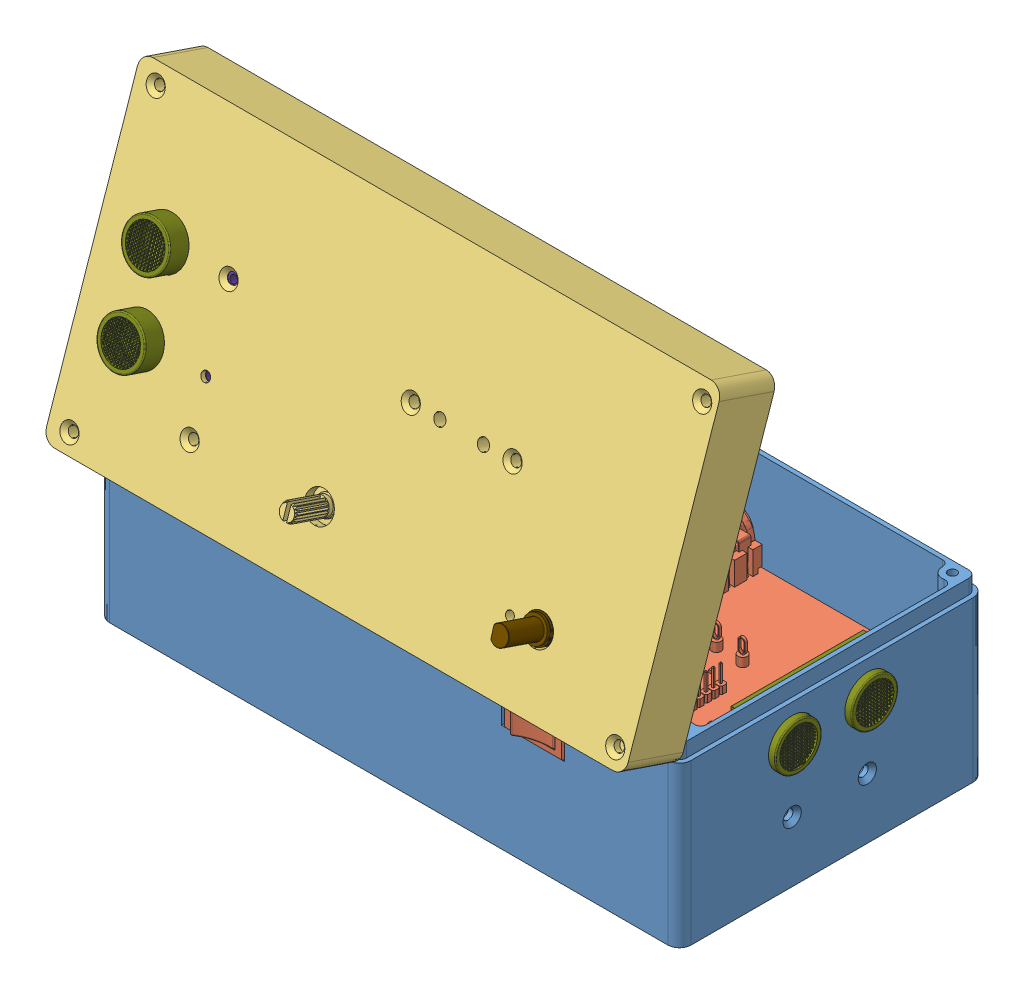
SolidWorks assembly Assemblage_Theremin, configuration Default. Lengths in mm.
Overall size (203.87 162.26 138.46).
66 component instances, 21 part files, 15 mates.
Components (placement in the parent):
- Theremin-Boitier_JonathanCHAFLA-1: Theremin-Boitier_JonathanCHAFLA [Default] at (-1328.4654 62.0969 1104.789) size (203 60 108)
- Theremin_PCB-Chafla.step-2: Theremin_PCB-Chafla.step [Default] at (-1384.7495 88.7032 1147.6303) x (1 0 0) z (0 1 0) size (155 102.12 38.23)
- Theremin-Boitier_JonathanCHAFLA-Couvercle-1: Theremin-Boitier_JonathanCHAFLA-Couvercle [Default] at (-1327.4934 174.761 1150.8521) x (1 0 0) z (0 0.946636 -0.322305) size (203 20 108)
- ThereminPart2_new.step-1: ThereminPart2_new.step [Default] at (-1282.4784 181.7259 1137.917) x (-0.999986 -0.005004 0.001704) z (0 0.322305 0.946636) size (85.91 17.79 19.44)
- PCB_Sensor_V3.step-1: PCB_Sensor_V3.step [Default] at (-1376.0149 146.0045 1153.5546) x (1 0 0) z (0 0.322305 0.946636) size (44.5 45.45 20.31)
  - Board.step-1: Board.step [Default] at origin size (24.5 45 1.61)
    - Open CASCADE STEP translator 6.8 1.1.1.step-1: Open CASCADE STEP translator 6.8 1.1.1.step [Default] at (0 0 -1.6063) size (24.5 45 1.61)
  - X1.step-1: X1.step [Default] at origin size (8.5 10.8 2.5)
    - 6023732704.step-1: 6023732704.step [Default] at (4.275 22.5 1.75) size (8.5 10.8 0.75)
      - Extruded.step-1: Extruded.step [Default] at origin size (8.5 10.8 0.75)
    - 6023732704.step-2: 6023732704.step [Default] at (4.275 22.5 0) size (8.5 10.8 0.75)
      - Extruded.step-1: Extruded.step [Default] at origin size (8.5 10.8 0.75)
    - 6023731264.step-1: 6023731264.step [Default] at (3.925 22.5 0.75) size (7.8 10.8 1)
      - Extruded-1.step-1: Extruded-1.step [Default] at origin size (7.8 10.8 1)
  - X2.step-1: X2.step [Default] at origin size (6.5 8.6 2.25)
    - 686104148922.step-1: 686104148922.step [Default] at (20.5501 22.4999 1.17) x (0 1 0) z (0 0 1) size (8.6 6.5 2.25)
      - 686104148922-0.step-1: 686104148922-0.step [Default] at origin size (8.6 4.5 2.2)
      - 6861xx148922_Patte.step-1: 6861xx148922_Patte.step [Default] at (2.9 0.7 -0.125) x (-1 0 0) z (0 0 1) size (1.4 3.1 1.85)
      - 6861xx148922_Patte2.step-1: 6861xx148922_Patte2.step [Default] at (-3.1 0.7 -0.125) x (-1 0 0) z (0 0 1) size (1.4 3.1 1.85)
      - 6861xx148922_Pin.step-1: 6861xx148922_Pin.step [Default] at (1.6 1.125 0.2986) x (-1 0 0) z (0 0 -1) size (0.2 4.6 2.25)
      - 6861xx148922_Pin.step-2: 6861xx148922_Pin.step [Default] at (0.6 1.125 0.2986) x (-1 0 0) z (0 0 -1) size (0.2 4.6 2.25)
      - 6861xx148922_Pin.step-3: 6861xx148922_Pin.step [Default] at (-0.4 1.125 0.2986) x (-1 0 0) z (0 0 -1) size (0.2 4.6 2.25)
      - 6861xx148922_Pin.step-4: 6861xx148922_Pin.step [Default] at (-1.4 1.125 0.2986) x (-1 0 0) z (0 0 -1) size (0.2 4.6 2.25)
      - 686104148922_Actuator.step-1: 686104148922_Actuator.step [Default] at (0 -2.25 0.4) x (1 0 0) z (0 -1 0) size (8.6 1.4 2.9)
  - C1.step-1: C1.step [Default] at origin size (1.25 2.01 0.94)
    - Cap_AVX_0805YA0R5BAT2A_eec.step-1: Cap_AVX_0805YA0R5BAT2A_eec.step [Default] at (13.5 18 0) x (0 1 0) z (0 0 1) size (2.01 1.25 0.94)
      - Terminals.step-1: Terminals.step [Default] at origin size (2.01 1.25 0.94)
      - Electrode.step-1: Electrode.step [Default] at origin size (1.01 1.25 0.94)
      - AVX.step-1: AVX.step [Default] at origin size (0.37 0.13 0)
  - Free-Models.step-1: Free-Models.step [Default] at origin size (35.25 45.45 20.1)
    - HC-SR04-UltrasonicSensor_v7.step-1: HC-SR04-UltrasonicSensor_v7.step [Default] at (-10 22.5 5.1) x (0 1 0) z (0 0 1) size (45.45 26.2 17.79)
    - 9774100360R_(rev1).step-1: 9774100360R_(rev1).step [Default] at (12.25 9.5 10) x (1 0 0) z (0 1 0) size (6 11.4 6)
    - 9774100360R_(rev1).step-2: 9774100360R_(rev1).step [Default] at (12.25 35.4279 10) x (1 0 0) z (0 1 0) size (6 11.4 6)
- PCB_Sensor_V3 - Copie.step-1: PCB_Sensor_V3 - Copie.step [Default] at (-1223.7904 95.1093 1125.4125) x (0 -1 0.00035) z (1 0 0) size (44.5 45.45 20.31)
  - Board.step-1: Board.step [Default] at origin size (24.5 45 1.61)
    - Open CASCADE STEP translator 6.8 1.1.1.step-1: Open CASCADE STEP translator 6.8 1.1.1.step [Default] at (0 0 -1.6063) size (24.5 45 1.61)
  - X1.step-1: X1.step [Default] at origin size (8.5 10.8 2.5)
    - 6023732704.step-1: 6023732704.step [Default] at (4.275 22.5 1.75) size (8.5 10.8 0.75)
      - Extruded.step-1: Extruded.step [Default] at origin size (8.5 10.8 0.75)
    - 6023732704.step-2: 6023732704.step [Default] at (4.275 22.5 0) size (8.5 10.8 0.75)
      - Extruded.step-1: Extruded.step [Default] at origin size (8.5 10.8 0.75)
    - 6023731264.step-1: 6023731264.step [Default] at (3.925 22.5 0.75) size (7.8 10.8 1)
      - Extruded-1.step-1: Extruded-1.step [Default] at origin size (7.8 10.8 1)
  - X2.step-1: X2.step [Default] at origin size (6.5 8.6 2.25)
    - 686104148922.step-1: 686104148922.step [Default] at (20.5501 22.4999 1.17) x (0 1 0) z (0 0 1) size (8.6 6.5 2.25)
      - 686104148922-0.step-1: 686104148922-0.step [Default] at origin size (8.6 4.5 2.2)
      - 6861xx148922_Patte.step-1: 6861xx148922_Patte.step [Default] at (2.9 0.7 -0.125) x (-1 0 0) z (0 0 1) size (1.4 3.1 1.85)
      - 6861xx148922_Patte2.step-1: 6861xx148922_Patte2.step [Default] at (-3.1 0.7 -0.125) x (-1 0 0) z (0 0 1) size (1.4 3.1 1.85)
      - 6861xx148922_Pin.step-1: 6861xx148922_Pin.step [Default] at (1.6 1.125 0.2986) x (-1 0 0) z (0 0 -1) size (0.2 4.6 2.25)
      - 6861xx148922_Pin.step-2: 6861xx148922_Pin.step [Default] at (0.6 1.125 0.2986) x (-1 0 0) z (0 0 -1) size (0.2 4.6 2.25)
      - 6861xx148922_Pin.step-3: 6861xx148922_Pin.step [Default] at (-0.4 1.125 0.2986) x (-1 0 0) z (0 0 -1) size (0.2 4.6 2.25)
      - 6861xx148922_Pin.step-4: 6861xx148922_Pin.step [Default] at (-1.4 1.125 0.2986) x (-1 0 0) z (0 0 -1) size (0.2 4.6 2.25)
      - 686104148922_Actuator.step-1: 686104148922_Actuator.step [Default] at (0 -2.25 0.4) x (1 0 0) z (0 -1 0) size (8.6 1.4 2.9)
  - C1.step-1: C1.step [Default] at origin size (1.25 2.01 0.94)
    - Cap_AVX_0805YA0R5BAT2A_eec.step-1: Cap_AVX_0805YA0R5BAT2A_eec.step [Default] at (13.5 18 0) x (0 1 0) z (0 0 1) size (2.01 1.25 0.94)
      - Terminals.step-1: Terminals.step [Default] at origin size (2.01 1.25 0.94)
      - Electrode.step-1: Electrode.step [Default] at origin size (1.01 1.25 0.94)
      - AVX.step-1: AVX.step [Default] at origin size (0.37 0.13 0)
  - Free-Models.step-1: Free-Models.step [Default] at origin size (35.25 45.45 20.1)
    - HC-SR04-UltrasonicSensor_v7.step-1: HC-SR04-UltrasonicSensor_v7.step [Default] at (-10 22.5 5.1) x (0 1 0) z (0 0 1) size (45.45 26.2 17.79)
    - 9774100360R_(rev1).step-1: 9774100360R_(rev1).step [Default] at (12.25 9.5 10) x (1 0 0) z (0 1 0) size (6 11.4 6)
    - 9774100360R_(rev1).step-2: 9774100360R_(rev1).step [Default] at (12.25 35.4279 10) x (1 0 0) z (0 1 0) size (6 11.4 6)
- A10405RNZQE_PART1.par-1: A10405RNZQE_PART1.par [Default] at (-1244.4868 141.1795 1153.1092) x (-0.999101 -0.04013 0.013663) z (-0.042392 0.945785 -0.322015) size (26.31 41.71 26.31)
- HP-2: HP [Défaut] at (-1406.4637 94.0969 1104.789) x (0 0 -1) z (1 0 0) size (36 36 16.5)
- jw-s11rww-2: jw-s11rww [Default] at (-1257.7609 105.7894 1152.6396) x (0 -1 0) z (0 0 1) size (15 22 25.64)
- Potentiometer-2: Potentiometer [Default] at (-1319.5713 140.814 1155.6071) x (-1 -0.000493 0.000168) z (-0.000521 0.946636 -0.322305) size (16.35 29.13 24.85)
Mates (geometry in assembly coordinates):
- Coïncidente20: coincident aligned: circle of Theremin-Boitier_JonathanCHAFLA-1; cylinder of PCB_Sensor_V3 - Copie.step-1/Free-Models.step-1/HC-SR04-UltrasonicSensor_v7.step-1 through (-1217.0904 105.0969 1089.789) axis (1 0 0) radius 8
- Coïncidente41: coincident aligned: plane of Theremin-Boitier_JonathanCHAFLA-1 through (-1378.4654 87.0969 1141.789) normal (0 1 0); circle of Theremin_PCB-Chafla.step-2
- Coïncidente76: coincident anti-aligned: line of Theremin-Boitier_JonathanCHAFLA-1 through (-1403.4637 117.0969 1154.6396) axis (1 0 0); line of Theremin-Boitier_JonathanCHAFLA-Couvercle-1 through (-1211.4637 117.0969 1154.6396) axis (-1 0 0)
- Coïncidente77: coincident aligned: plane of Theremin-Boitier_JonathanCHAFLA-1 through (-1207.4637 122.0969 1049.6396) normal (1 0 0); plane of Theremin-Boitier_JonathanCHAFLA-Couvercle-1 through (-1207.4637 123.5429 1173.5723) normal (1 0 0)
- Coïncidente78: coincident aligned: cylinder of Theremin-Boitier_JonathanCHAFLA-Couvercle-1 through (-1386.0149 158.6582 1161.6165) axis (0 -0.322305 -0.946636) radius 8; circle of PCB_Sensor_V3.step-1/Free-Models.step-1/HC-SR04-UltrasonicSensor_v7.step-1
- Coïncidente79: coincident anti-aligned: circle of Theremin-Boitier_JonathanCHAFLA-Couvercle-1; circle of PCB_Sensor_V3.step-1/Free-Models.step-1/HC-SR04-UltrasonicSensor_v7.step-1
- Coïncidente80: coincident aligned: circle of Theremin-Boitier_JonathanCHAFLA-Couvercle-1; plane of Potentiometer-1 through (-1320.2674 145.4627 1160.4306) normal (0 0.336561 0.941662)
- Coïncidente82: coincident aligned: circle of Theremin-Boitier_JonathanCHAFLA-Couvercle-1; plane of ThereminPart2_new.step-1 through (-1299.9385 177.7616 1149.8304) normal (0 0.322305 0.946636)
- Coaxiale41: concentric aligned: cylinder of Theremin-Boitier_JonathanCHAFLA-Couvercle-1 through (-1299.9385 179.3732 1154.5636) axis (0 -0.322305 -0.946636) radius 1.8; cylinder of ThereminPart2_new.step-1 through (-1299.9385 175.6989 1143.7719) axis (0 -0.322305 -0.946636) radius 3
- Coïncidente86: coincident aligned: circle of Theremin-Boitier_JonathanCHAFLA-Couvercle-1; plane of A10405RNZQE_PART1.par-1 through (-1244.4868 143.9793 1161.3324) normal (0 0.322305 0.946636)
- Coïncidente88: coincident anti-aligned: circle of Theremin-Boitier_JonathanCHAFLA-Couvercle-1; plane of Potentiometer-2 through (-1319.5713 142.8896 1161.7034) normal (0 -0.322305 -0.946636)
- Coaxiale48: concentric aligned: circle of Theremin-Boitier_JonathanCHAFLA-Couvercle-1; circle of Potentiometer-2
- Coïncidente90: coincident aligned: line of Theremin-Boitier_JonathanCHAFLA-1 through (-1268.6403 98.9894 1154.6396) axis (1 0 0); line of jw-s11rww-2 through (-1267.3488 98.9894 1154.6396) axis (1 0 0)
- Coïncidente92: coincident aligned: cylinder of Theremin-Boitier_JonathanCHAFLA-1 through (-1407.4637 94.0969 1104.789) axis (1 0 0) radius 18; circle of HP-2
- Coïncidente93: coincident aligned: circle of Theremin-Boitier_JonathanCHAFLA-1; circle of HP-2
